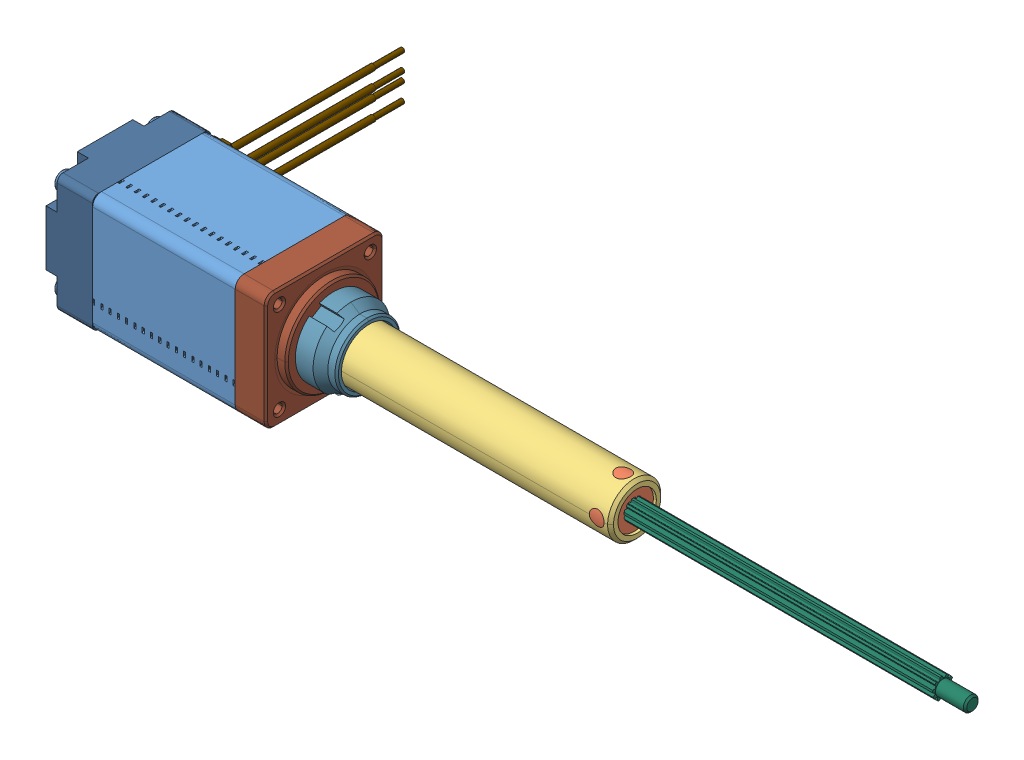
SolidWorks assembly 20K-2M..50, configuration 默认. Lengths in mm.
Overall size (146.95 25.88 47.14).
32 component instances, 21 part files, 0 mates.
Components (placement in the parent):
- 20K-2M..50.STEP-1: 20K-2M..50.STEP [默认] at origin size (146.95 25.88 47.14)
  - 02-20-42.STEP-1: 02-20-42.STEP [默认] at (19.975 0 0) x (0 -1 0) z (-1 0 0) size (25.88 26.04 31.85)
    - 02-20-24.15_10-20-001-2.STEP-1: 02-20-24.15_10-20-001-2.STEP [默认] at origin size (20 20 24.15)
    - 13-20-12.5____.STEP-1: 13-20-12.5____.STEP [默认] at (0 0 16.075) x (-1 0 0) z (0 0 -1) size (18.2 22.2 16.51)
    - 13-20-12.5______.STEP-1: 13-20-12.5______.STEP [默认] at (0 0 -14.575) x (0.707107 0.707107 0) z (0 0 1) size (18.3 18.3 15.8)
    - 20-20__________.STEP-1: 20-20__________.STEP [默认] at (0 0 15.675) size (17.8 21 0.9)
    - 13-20-001________.STEP-1: 13-20-001________.STEP [默认] at (0 -8.6 12.175) x (1 0 0) z (0 0 -1) size (10.5 7.2 3.5)
  - 03-20-006____42_____default.STEP-1: 03-20-006____42_____default.STEP [默认] at (5.7 0 0) x (1 0 0) z (0 0.381126 -0.924523) size (29.65 16.26 16.27)
    - 06-20-006____42______YK_01-20-007-1.STEP-1: 06-20-006____42______YK_01-20-007-1.STEP [默认] at origin size (29.65 7 7)
    - 03-20-4.2-6YK_10-20-006-2.STEP-1: 03-20-4.2-6YK_10-20-006-2.STEP [默认] at (22.53 0 0) x (0 0.91534 0.402682) z (-1 0 0) size (12.06 12.08 4.2)
    - 10-20-001__________.STEP-1: 10-20-001__________.STEP [默认] at (14.67 0 0) x (0 0 1) z (-1 0 0) size (11.2 11.2 1.3)
    - 08-20-001_____07-20-001-1.STEP-1: 08-20-001_____07-20-001-1.STEP [默认] at (20.41 0 0) x (0 0 1) z (-1 0 0) size (11 11 1.5)
    - 08-20-001_____07-20-001-1.STEP-2: 08-20-001_____07-20-001-1.STEP [默认] at (9.43 0 0) x (0 0 1) z (-1 0 0) size (11 11 1.5)
    - 03-20-4.2-6YK_10-20-006-2.STEP-2: 03-20-4.2-6YK_10-20-006-2.STEP [默认] at (16.79 0 0) x (0 0.888249 0.459362) z (-1 0 0) size (12.06 12.08 4.2)
    - 03-20-4.2-6YK_10-20-006-2.STEP-3: 03-20-4.2-6YK_10-20-006-2.STEP [默认] at (11.55 0 0) x (0 0.91534 0.402682) z (-1 0 0) size (12.06 12.08 4.2)
    - 03-20-4.2-6YK_10-20-006-2.STEP-4: 03-20-4.2-6YK_10-20-006-2.STEP [默认] at (5.81 0 0) x (0 0.888249 0.459362) z (-1 0 0) size (12.06 12.08 4.2)
  - 01-20-006__20__________YK__.STEP-1: 01-20-006__20__________YK__.STEP [默认] at origin size (8.8 20 20)
  - 01-20-005(20____________YK__.STEP-1: 01-20-005(20____________YK__.STEP [默认] at (31.25 0 0) x (0 0 -1) z (1 0 0) size (20 20 7.5)
  - 09-20-001____9X__5X4)_09-20-001.STEP-1: 09-20-001____9X__5X4)_09-20-001.STEP [默认] at (5.7 0 0) x (1 0 0) z (0 0.998527 -0.054257) size (3 9 9)
  - 09-20-001____9X__5X4)_09-20-001.STEP-2: 09-20-001____9X__5X4)_09-20-001.STEP [默认] at (32.35 0 0) x (1 0 0) z (0 0.945037 0.326964) size (3 9 9)
  - 06-20-017__20________YK___20____________YK.STEP-1: 06-20-017__20________YK___20____________YK.STEP [默认] at (30.35 0 0) x (0 0.924523 0.381126) z (-1 0 0) size (6.01 6.01 10)
  - 07-20-007__________________.STEP-1: 07-20-007__________________.STEP [默认] at (38.75 0 0) x (-1 0 0) z (0 -0.999857 -0.016895) size (6 12.92 13)
  - 07-20-015-1______________.STEP-1: 07-20-015-1______________.STEP [默认] at (82.15 0 0) x (0 -0.714016 0.700129) z (1 0 0) size (3.42 3.5 64.8)
  - 07-20-015-2______________.STEP-1: 07-20-015-2______________.STEP [默认] at (20.35 0 0) x (0 0.924225 0.381849) z (1 0 0) size (3.5 3.9 64.81)
  - 07-20-006__20______.STEP-1: 07-20-006__20______.STEP [默认] at (86.15 0 0) x (0 0.924225 0.381849) z (1 0 0) size (4.8 4.8 0.5)
  - 14-20-001__20-28____________________.STEP-1: 14-20-001__20-28____________________.STEP [默认] at (6.48 -0.2 -10) x (0 -1 0) z (0 0 1) size (10.5 3.4 24.5)
  - 11-20-001__M2-24.5__20-30__.STEP-1: 11-20-001__M2-24.5__20-30__.STEP [默认] at (0.39 7.7 -7.7) x (0 -0.010787 -0.999942) z (1 0 0) size (3 3 26)
  - 11-20-001__M2-24.5__20-30__.STEP-2: 11-20-001__M2-24.5__20-30__.STEP [默认] at (0.39 7.7 7.7) x (0 0.999942 -0.010787) z (1 0 0) size (3 3 26)
  - 11-20-001__M2-24.5__20-30__.STEP-3: 11-20-001__M2-24.5__20-30__.STEP [默认] at (0.39 -7.7 7.7) x (0 0.010787 0.999942) z (1 0 0) size (3 3 26)
  - 11-20-001__M2-24.5__20-30__.STEP-4: 11-20-001__M2-24.5__20-30__.STEP [默认] at (0.39 -7.7 -7.7) x (0 -0.999942 0.010787) z (1 0 0) size (3 3 26)
  - 07-20-002__20________________.STEP-1: 07-20-002__20________________.STEP [默认] at (87.8 0 0) x (0 0 -1) z (1 0 0) size (9.01 9.01 3.1)
  - 07-20-015-3__20_____________08-20-002-1.STEP-1: 07-20-015-3__20_____________08-20-002-1.STEP [默认] at (35.35 0 0) x (0 0 -1) z (1 0 0) size (9.01 9.01 54.8)
